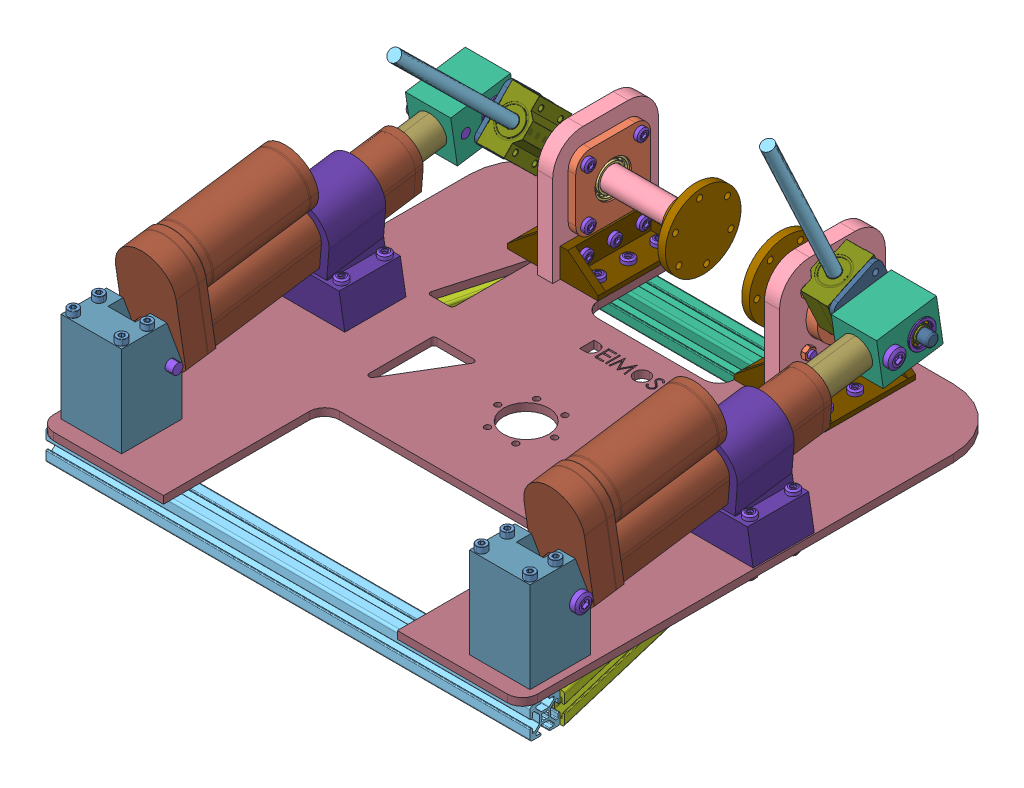
SolidWorks assembly Arm_base_2025_Final, configuration Default. Lengths in mm.
Overall size (325.65 204.06 325).
175 component instances, 27 part files, 250 mates.
Components (placement in the parent):
- linnear rod coupler-1: linnear rod coupler [Default] at (190.8714 137.6403 148.5796) x (0 0.712121 -0.702057) z (-1 0 0) size (18.5 18.5 20.01)
- base bearing assambly-1: base bearing assambly [Default] at (234.6957 114.573 126.7936) x (0 0 1) z (-1 0 0) size (49.5 49.5 22)
  - base shaft bearing housing-1: base shaft bearing housing [Default] at (21.786 23.0673 38.1242) size (49.5 49.5 22)
  - 61802  15x24x5mm-1: 61802  15x24x5mm [Default] at (21.786 23.0673 37.1242) x (0 0 -1) z (1 0 0) size (5 24 24)
  - 61802  15x24x5mm-2: 61802  15x24x5mm [Default] at (21.786 23.0673 22.1242) x (0 0 -1) z (1 0 0) size (5 24 24)
- V8_bearing holder holderURC 2024_V4-1: V8_bearing holder holderURC 2024_V4 [Default] at (213.5714 172.6403 113.5796) x (0 0 1) z (-1 0 0) size (70 80 10)
- linear guid rod-1: linear guid rod [Default] at (184.8714 141.8526 152.8523) x (0.966938 -0.1816 0.179034) z (-0.255013 -0.688576 0.678846) size (8 150 8)
- Connector to Linear bearing-1: Connector to Linear bearing [Default] at (123.1767 129.7873 154.7447) x (1 0 0) z (0 0.553629 0.832764) size (32.2 49.07 49.79)
  - V8_connectorURC 2024_V4-1: V8_connectorURC 2024_V4 [Default] at (40.3948 35.6094 31.6737) x (0 -0.66999 0.74237) z (-1 0 0) size (40 30 30)
  - V8_F688ZZ_assemblyURC 2024_V4-1: V8_F688ZZ_assemblyURC 2024_V4 [Default] at (41.4948 16.099 30.9035) x (0 1 0) z (0 0 1) size (20.89 5 20.89)
    - V8_F688ZZ_shaftURC 2024_V4-1: V8_F688ZZ_shaftURC 2024_V4 [Default] at origin size (10.7 5 10.7)
    - V8_F688ZZ_HousingURC 2024_V4-1: V8_F688ZZ_HousingURC 2024_V4 [Default] x (0.984312 0 0.176438) z (-0.176438 0 0.984312) size (18 5 18)
    - V8_F688ZZ_BallURC 2024_V4-1: V8_F688ZZ_BallURC 2024_V4 [Default] at (5.5752 2.5 -2.1489) x (0.959238 0.232099 0.161224) z (-0.142462 -0.095558 0.985177) size (2 2 2)
    - V8_F688ZZ_BallURC 2024_V4-20: V8_F688ZZ_BallURC 2024_V4 [Default] at (3.2474 2.5 -5.0155) x (0.870805 0.232099 -0.433393) z (0.463818 -0.095558 0.880762) size (2 2 2)
    - V8_F688ZZ_BallURC 2024_V4-21: V8_F688ZZ_BallURC 2024_V4 [Default] at (-0.3209 2.5 -5.9664) x (0.449753 0.232099 -0.862469) z (0.892936 -0.095558 0.439926) size (2 2 2)
    - V8_F688ZZ_BallURC 2024_V4-22: V8_F688ZZ_BallURC 2024_V4 [Default] at (-3.7665 2.5 -4.6383) x (-0.143088 0.232099 -0.96211) z (0.980982 -0.095558 -0.168947) size (2 2 2)
    - V8_F688ZZ_BallURC 2024_V4-23: V8_F688ZZ_BallURC 2024_V4 [Default] at (-5.7735 2.5 -1.5385) x (-0.681275 0.232099 -0.694258) z (0.694326 -0.095558 -0.713288) size (2 2 2)
    - V8_F688ZZ_BallURC 2024_V4-24: V8_F688ZZ_BallURC 2024_V4 [Default] at (-5.5752 2.5 2.1489) x (-0.959238 0.232099 -0.161224) z (0.142462 -0.095558 -0.985177) size (2 2 2)
    - V8_F688ZZ_BallURC 2024_V4-25: V8_F688ZZ_BallURC 2024_V4 [Default] at (-3.2474 2.5 5.0155) x (-0.870805 0.232099 0.433393) z (-0.463818 -0.095558 -0.880762) size (2 2 2)
    - V8_F688ZZ_BallURC 2024_V4-26: V8_F688ZZ_BallURC 2024_V4 [Default] at (0.3209 2.5 5.9664) x (-0.449753 0.232099 0.862469) z (-0.892936 -0.095558 -0.439926) size (2 2 2)
    - V8_F688ZZ_BallURC 2024_V4-27: V8_F688ZZ_BallURC 2024_V4 [Default] at (3.7665 2.5 4.6383) x (0.143088 0.232099 0.96211) z (-0.980982 -0.095558 0.168947) size (2 2 2)
    - V8_F688ZZ_BallURC 2024_V4-28: V8_F688ZZ_BallURC 2024_V4 [Default] at (5.7735 2.5 1.5385) x (0.681275 0.232099 0.694258) z (-0.694326 -0.095558 0.713288) size (2 2 2)
  - V8_F688ZZ_assemblyURC 2024_V4-2: V8_F688ZZ_assemblyURC 2024_V4 [Default] at (9.2948 16.099 30.9035) x (0 -0.381849 0.924225) z (0 0.924225 0.381849) size (20.89 5 20.89)
    - V8_F688ZZ_shaftURC 2024_V4-1: V8_F688ZZ_shaftURC 2024_V4 [Default] at origin size (10.7 5 10.7)
    - V8_F688ZZ_HousingURC 2024_V4-1: V8_F688ZZ_HousingURC 2024_V4 [Default] x (0.984312 0 0.176438) z (-0.176438 0 0.984312) size (18 5 18)
    - V8_F688ZZ_BallURC 2024_V4-1: V8_F688ZZ_BallURC 2024_V4 [Default] at (5.5752 2.5 -2.1489) x (0.959238 0.232099 0.161224) z (-0.142462 -0.095558 0.985177) size (2 2 2)
    - V8_F688ZZ_BallURC 2024_V4-20: V8_F688ZZ_BallURC 2024_V4 [Default] at (3.2474 2.5 -5.0155) x (0.870805 0.232099 -0.433393) z (0.463818 -0.095558 0.880762) size (2 2 2)
    - V8_F688ZZ_BallURC 2024_V4-21: V8_F688ZZ_BallURC 2024_V4 [Default] at (-0.3209 2.5 -5.9664) x (0.449753 0.232099 -0.862469) z (0.892936 -0.095558 0.439926) size (2 2 2)
    - V8_F688ZZ_BallURC 2024_V4-22: V8_F688ZZ_BallURC 2024_V4 [Default] at (-3.7665 2.5 -4.6383) x (-0.143088 0.232099 -0.96211) z (0.980982 -0.095558 -0.168947) size (2 2 2)
    - V8_F688ZZ_BallURC 2024_V4-23: V8_F688ZZ_BallURC 2024_V4 [Default] at (-5.7735 2.5 -1.5385) x (-0.681275 0.232099 -0.694258) z (0.694326 -0.095558 -0.713288) size (2 2 2)
    - V8_F688ZZ_BallURC 2024_V4-24: V8_F688ZZ_BallURC 2024_V4 [Default] at (-5.5752 2.5 2.1489) x (-0.959238 0.232099 -0.161224) z (0.142462 -0.095558 -0.985177) size (2 2 2)
    - V8_F688ZZ_BallURC 2024_V4-25: V8_F688ZZ_BallURC 2024_V4 [Default] at (-3.2474 2.5 5.0155) x (-0.870805 0.232099 0.433393) z (-0.463818 -0.095558 -0.880762) size (2 2 2)
    - V8_F688ZZ_BallURC 2024_V4-26: V8_F688ZZ_BallURC 2024_V4 [Default] at (0.3209 2.5 5.9664) x (-0.449753 0.232099 0.862469) z (-0.892936 -0.095558 -0.439926) size (2 2 2)
    - V8_F688ZZ_BallURC 2024_V4-27: V8_F688ZZ_BallURC 2024_V4 [Default] at (3.7665 2.5 4.6383) x (0.143088 0.232099 0.96211) z (-0.980982 -0.095558 0.168947) size (2 2 2)
    - V8_F688ZZ_BallURC 2024_V4-28: V8_F688ZZ_BallURC 2024_V4 [Default] at (5.7735 2.5 1.5385) x (0.681275 0.232099 0.694258) z (-0.694326 -0.095558 0.713288) size (2 2 2)
- V8_bearing and cam connection_for_v4URC 2024_V4 laser cut-1: V8_bearing and cam connection_for_v4URC 2024_V4 laser cut [Default] at (170.6714 137.31 173.1714) x (0 0.702057 0.712121) z (1 0 0) size (30 35 48)
- V8_LA_Body_V4-1: V8_LA_Body_V4 [Default] at (148.5714 135.8868 383.5572) x (0 -0.989144 -0.146946) z (-1 0 0) size (74 184 40)
- V8_LA_RodURC 2024_V4-1: V8_LA_RodURC 2024_V4 [Default] at (148.5714 158.4515 184.0304) x (1 0 0) z (0 -0.989144 -0.146946) size (20 121 20)
- V8_base plate for LAURC 2024_V4-1: V8_base plate for LAURC 2024_V4 [Default] at (283.5714 87.6403 412.2334) x (0 0 -1) z (0 1 0) size (325 320 5)
- LA_back holder-1: LA_back holder [Default] at (148.5714 152.6403 403.5796) x (-1 0 0) z (0 0 -1) size (40 60 40)
- Connector to Linear bearing-2: Connector to Linear bearing [Default] at (393.1767 131.5103 143.1465) x (1 0 0) z (0 0.553629 0.832764) size (32.2 49.07 49.79)
  - V8_connectorURC 2024_V4-1: V8_connectorURC 2024_V4 [Default] at (40.3948 35.6094 31.6737) x (0 -0.66999 0.74237) z (-1 0 0) size (40 30 30)
  - V8_F688ZZ_assemblyURC 2024_V4-1: V8_F688ZZ_assemblyURC 2024_V4 [Default] at (41.4948 16.099 30.9035) x (0 1 0) z (0 0 1) size (20.89 5 20.89)
    - V8_F688ZZ_shaftURC 2024_V4-1: V8_F688ZZ_shaftURC 2024_V4 [Default] at origin size (10.7 5 10.7)
    - V8_F688ZZ_HousingURC 2024_V4-1: V8_F688ZZ_HousingURC 2024_V4 [Default] x (0.984312 0 0.176438) z (-0.176438 0 0.984312) size (18 5 18)
    - V8_F688ZZ_BallURC 2024_V4-1: V8_F688ZZ_BallURC 2024_V4 [Default] at (5.5752 2.5 -2.1489) x (0.959238 0.232099 0.161224) z (-0.142462 -0.095558 0.985177) size (2 2 2)
    - V8_F688ZZ_BallURC 2024_V4-20: V8_F688ZZ_BallURC 2024_V4 [Default] at (3.2474 2.5 -5.0155) x (0.870805 0.232099 -0.433393) z (0.463818 -0.095558 0.880762) size (2 2 2)
    - V8_F688ZZ_BallURC 2024_V4-21: V8_F688ZZ_BallURC 2024_V4 [Default] at (-0.3209 2.5 -5.9664) x (0.449753 0.232099 -0.862469) z (0.892936 -0.095558 0.439926) size (2 2 2)
    - V8_F688ZZ_BallURC 2024_V4-22: V8_F688ZZ_BallURC 2024_V4 [Default] at (-3.7665 2.5 -4.6383) x (-0.143088 0.232099 -0.96211) z (0.980982 -0.095558 -0.168947) size (2 2 2)
    - V8_F688ZZ_BallURC 2024_V4-23: V8_F688ZZ_BallURC 2024_V4 [Default] at (-5.7735 2.5 -1.5385) x (-0.681275 0.232099 -0.694258) z (0.694326 -0.095558 -0.713288) size (2 2 2)
    - V8_F688ZZ_BallURC 2024_V4-24: V8_F688ZZ_BallURC 2024_V4 [Default] at (-5.5752 2.5 2.1489) x (-0.959238 0.232099 -0.161224) z (0.142462 -0.095558 -0.985177) size (2 2 2)
    - V8_F688ZZ_BallURC 2024_V4-25: V8_F688ZZ_BallURC 2024_V4 [Default] at (-3.2474 2.5 5.0155) x (-0.870805 0.232099 0.433393) z (-0.463818 -0.095558 -0.880762) size (2 2 2)
    - V8_F688ZZ_BallURC 2024_V4-26: V8_F688ZZ_BallURC 2024_V4 [Default] at (0.3209 2.5 5.9664) x (-0.449753 0.232099 0.862469) z (-0.892936 -0.095558 -0.439926) size (2 2 2)
    - V8_F688ZZ_BallURC 2024_V4-27: V8_F688ZZ_BallURC 2024_V4 [Default] at (3.7665 2.5 4.6383) x (0.143088 0.232099 0.96211) z (-0.980982 -0.095558 0.168947) size (2 2 2)
    - V8_F688ZZ_BallURC 2024_V4-28: V8_F688ZZ_BallURC 2024_V4 [Default] at (5.7735 2.5 1.5385) x (0.681275 0.232099 0.694258) z (-0.694326 -0.095558 0.713288) size (2 2 2)
  - V8_F688ZZ_assemblyURC 2024_V4-2: V8_F688ZZ_assemblyURC 2024_V4 [Default] at (9.2948 16.099 30.9035) x (0 -0.381849 0.924225) z (0 0.924225 0.381849) size (20.89 5 20.89)
    - V8_F688ZZ_shaftURC 2024_V4-1: V8_F688ZZ_shaftURC 2024_V4 [Default] at origin size (10.7 5 10.7)
    - V8_F688ZZ_HousingURC 2024_V4-1: V8_F688ZZ_HousingURC 2024_V4 [Default] x (0.984312 0 0.176438) z (-0.176438 0 0.984312) size (18 5 18)
    - V8_F688ZZ_BallURC 2024_V4-1: V8_F688ZZ_BallURC 2024_V4 [Default] at (5.5752 2.5 -2.1489) x (0.959238 0.232099 0.161224) z (-0.142462 -0.095558 0.985177) size (2 2 2)
    - V8_F688ZZ_BallURC 2024_V4-20: V8_F688ZZ_BallURC 2024_V4 [Default] at (3.2474 2.5 -5.0155) x (0.870805 0.232099 -0.433393) z (0.463818 -0.095558 0.880762) size (2 2 2)
    - V8_F688ZZ_BallURC 2024_V4-21: V8_F688ZZ_BallURC 2024_V4 [Default] at (-0.3209 2.5 -5.9664) x (0.449753 0.232099 -0.862469) z (0.892936 -0.095558 0.439926) size (2 2 2)
    - V8_F688ZZ_BallURC 2024_V4-22: V8_F688ZZ_BallURC 2024_V4 [Default] at (-3.7665 2.5 -4.6383) x (-0.143088 0.232099 -0.96211) z (0.980982 -0.095558 -0.168947) size (2 2 2)
    - V8_F688ZZ_BallURC 2024_V4-23: V8_F688ZZ_BallURC 2024_V4 [Default] at (-5.7735 2.5 -1.5385) x (-0.681275 0.232099 -0.694258) z (0.694326 -0.095558 -0.713288) size (2 2 2)
    - V8_F688ZZ_BallURC 2024_V4-24: V8_F688ZZ_BallURC 2024_V4 [Default] at (-5.5752 2.5 2.1489) x (-0.959238 0.232099 -0.161224) z (0.142462 -0.095558 -0.985177) size (2 2 2)
    - V8_F688ZZ_BallURC 2024_V4-25: V8_F688ZZ_BallURC 2024_V4 [Default] at (-3.2474 2.5 5.0155) x (-0.870805 0.232099 0.433393) z (-0.463818 -0.095558 -0.880762) size (2 2 2)
    - V8_F688ZZ_BallURC 2024_V4-26: V8_F688ZZ_BallURC 2024_V4 [Default] at (0.3209 2.5 5.9664) x (-0.449753 0.232099 0.862469) z (-0.892936 -0.095558 -0.439926) size (2 2 2)
    - V8_F688ZZ_BallURC 2024_V4-27: V8_F688ZZ_BallURC 2024_V4 [Default] at (3.7665 2.5 4.6383) x (0.143088 0.232099 0.96211) z (-0.980982 -0.095558 0.168947) size (2 2 2)
    - V8_F688ZZ_BallURC 2024_V4-28: V8_F688ZZ_BallURC 2024_V4 [Default] at (5.7735 2.5 1.5385) x (0.681275 0.232099 0.694258) z (-0.694326 -0.095558 0.713288) size (2 2 2)
- LA_back holder-2: LA_back holder [Default] at (418.5714 152.6403 403.5796) x (-1 0 0) z (0 0 -1) size (40 60 40)
- V8_bearing and cam connection_for_v4URC 2024_V4 laser cut-2: V8_bearing and cam connection_for_v4URC 2024_V4 laser cut [Default] at (396.4714 168.2112 182.1724) x (0 -0.906049 -0.423172) z (-1 0 0) size (30 35 48)
- V8_LA_RodURC 2024_V4-2: V8_LA_RodURC 2024_V4 [Default] at (418.5714 160.1745 172.4322) x (1 0 0) z (0 -0.989144 -0.146946) size (20 121 20)
- linnear rod coupler-2: linnear rod coupler [Default] at (376.2714 137.6403 148.5796) x (0 -0.423172 0.906049) z (1 0 0) size (18.5 18.5 20.01)
- lock_nut_for coupler-2: lock_nut_for coupler [Default] at (396.2714 137.6403 148.5796) x (0 -0.658716 -0.752392) z (1 0 0) size (18 18 13)
- linear guid rod-2: linear guid rod [Default] at (382.2714 133.5883 146.6871) x (0.37331 0.39258 -0.840548) z (0.927707 -0.157974 0.338237) size (8 150 8)
- base bearing assambly-2: base bearing assambly [Default] at (332.4472 114.573 170.3656) x (0 0 -1) z (1 0 0) size (49.5 49.5 22)
  - base shaft bearing housing-1: base shaft bearing housing [Default] at (21.786 23.0673 38.1242) size (49.5 49.5 22)
  - 61802  15x24x5mm-1: 61802  15x24x5mm [Default] at (21.786 23.0673 37.1242) x (0 0 -1) z (1 0 0) size (5 24 24)
  - 61802  15x24x5mm-2: 61802  15x24x5mm [Default] at (21.786 23.0673 22.1242) x (0 0 -1) z (1 0 0) size (5 24 24)
- V8_bearing holder holderURC 2024_V4-2: V8_bearing holder holderURC 2024_V4 [Default] at (353.5714 172.6403 183.5796) x (0 0 -1) z (1 0 0) size (70 80 10)
- V8_LA_Body_V4-2: V8_LA_Body_V4 [Default] at (418.5714 135.8868 383.5572) x (0 -0.989144 -0.146946) z (-1 0 0) size (74 184 40)
- linear bearing robotic arm-1: linear bearing robotic arm [Default] at (182.4393 149.7722 160.8854) x (0 0.712121 -0.702057) z (1 0 0) size (34 30.1 22.2)
- linear bearing robotic arm-2: linear bearing robotic arm [Default] at (384.7035 175.6167 166.3166) x (0 0.423172 -0.906049) z (-1 0 0) size (34 30.1 22.2)
- linear_acutator_holder-1: linear_acutator_holder [Default] at (418.6971 146.656 247.7322) x (0 -0.989144 -0.146946) z (0 -0.146946 0.989144) size (75.87 48 40)
- linear_acutator_holder-2: linear_acutator_holder [Default] at (148.6971 146.656 247.7322) x (0 -0.989144 -0.146946) z (0 -0.146946 0.989144) size (75.87 48 40)
- l bracket_arm base flang-1: l bracket_arm base flang [Default] at (363.5714 111.6403 178.5796) x (0 0 -1) z (1 0 0) size (60 19 25)
- l bracket_arm base flang-2: l bracket_arm base flang [Default] at (353.5714 111.6403 118.5796) x (0 0 1) z (-1 0 0) size (60 19 25)
- l bracket_arm base flang-3: l bracket_arm base flang [Default] at (203.5714 111.6403 118.5796) x (0 0 1) z (-1 0 0) size (60 19 25)
- l bracket_arm base flang-4: l bracket_arm base flang [Default] at (213.5714 111.6403 178.5796) x (0 0 -1) z (1 0 0) size (60 19 25)
- Screw_DIN_912_M4x70_A2.step-1: Screw_DIN_912_M4x70_A2.step [Default] at (402.5714 82.6403 419.5796) size (7 74 7)
- Screw_DIN_912_M4x70_A2.step-2: Screw_DIN_912_M4x70_A2.step [Default] at (434.5714 82.6403 419.5796) x (0.982082 0 -0.188455) z (0.188455 0 0.982082) size (7 74 7)
- Screw_DIN_912_M4x70_A2.step-4: Screw_DIN_912_M4x70_A2.step [Default] at (434.5714 82.6403 402.6026) x (0.918365 0 -0.395734) z (0.395734 0 0.918365) size (7 74 7)
- Screw_DIN_912_M4x70_A2.step-6: Screw_DIN_912_M4x70_A2.step [Default] at (402.5714 82.6403 402.6026) x (0.8 0 -0.6) z (0.6 0 0.8) size (7 74 7)
- Screw_DIN_912_M4x70_A2.step-8: Screw_DIN_912_M4x70_A2.step [Default] at (164.5714 82.6403 419.5796) x (0.63358 0 -0.773678) z (0.773678 0 0.63358) size (7 74 7)
- Screw_DIN_912_M4x70_A2.step-10: Screw_DIN_912_M4x70_A2.step [Default] at (164.5714 82.6403 402.6026) x (0.443629 0 -0.896211) z (0.896211 0 0.443629) size (7 74 7)
- Screw_DIN_912_M4x70_A2.step-12: Screw_DIN_912_M4x70_A2.step [Default] at (132.5714 82.6403 419.5796) x (0.263225 0 -0.964735) z (0.964735 0 0.263225) size (7 74 7)
- Screw_DIN_912_M4x70_A2.step-14: Screw_DIN_912_M4x70_A2.step [Default] at (132.5714 82.6403 402.6026) x (0.120178 0 -0.992752) z (0.992752 0 0.120178) size (7 74 7)
- hex nut style 1 gradeab_iso-8: hex nut style 1 gradeab_iso [ISO - 4032 - M4 - W - N] at (402.5714 84.4403 419.5796) x (0.999814 0 0.019309) z (0 -1 0) size (7 8.08 3.2)
- hex nut style 1 gradeab_iso-9: hex nut style 1 gradeab_iso [ISO - 4032 - M4 - W - N] at (434.5714 84.4403 419.5796) x (0.985538 0 -0.169457) z (0 -1 0) size (7 8.08 3.2)
- hex nut style 1 gradeab_iso-11: hex nut style 1 gradeab_iso [ISO - 4032 - M4 - W - N] at (434.5714 84.4403 402.6026) x (0.563007 0 -0.826452) z (0 -1 0) size (7 8.08 3.2)
- hex nut style 1 gradeab_iso-14: hex nut style 1 gradeab_iso [ISO - 4032 - M4 - W - N] at (402.5714 84.4403 402.6026) x (0.563007 0 -0.826452) z (0 -1 0) size (7 8.08 3.2)
- hex nut style 1 gradeab_iso-16: hex nut style 1 gradeab_iso [ISO - 4032 - M4 - W - N] at (164.5714 84.4403 419.5796) x (0.648401 0 -0.761299) z (0 -1 0) size (7 8.08 3.2)
- hex nut style 1 gradeab_iso-18: hex nut style 1 gradeab_iso [ISO - 4032 - M4 - W - N] at (164.5714 84.4403 402.6026) x (0.563007 0 -0.826452) z (0 -1 0) size (7 8.08 3.2)
- hex nut style 1 gradeab_iso-20: hex nut style 1 gradeab_iso [ISO - 4032 - M4 - W - N] at (132.5714 84.4403 419.5796) x (0.563007 0 -0.826452) z (0 -1 0) size (7 8.08 3.2)
- hex nut style 1 gradeab_iso-22: hex nut style 1 gradeab_iso [ISO - 4032 - M4 - W - N] at (132.5714 84.4403 402.6026) x (0.563007 0 -0.826452) z (0 -1 0) size (7 8.08 3.2)
- V8_shaftURC 2024_V4 real part-1: V8_shaftURC 2024_V4 real part [Default] at (378.5714 128.7575 141.4959) x (-1 0 0) z (0 0.623486 -0.781835) size (75.7 15 15)
- V8_shaftURC 2024_V4-1: V8_shaftURC 2024_V4 [Default] at (223.809 124.5508 145.7858) x (1 0 0) z (0 -0.208738 0.977971) size (115.2 15 15)
- 20 20 aluminium extrusion T slot-1: 20 20 aluminium extrusion T slot [Default] at (4123.5714 77.6403 418.5796) x (0 0 -1) z (-1 0 0) size (20 20 320)
- 20 20 aluminium extrusion T slot 200 mm-1: 20 20 aluminium extrusion T slot 200 mm [Default] at (4183.5714 77.6403 148.5796) x (0 0 -1) z (-1 0 0) size (20 20 200)
- 20 20 aluminium extrusion T slot at angle-1: 20 20 aluminium extrusion T slot at angle [Default] at (-494.3957 77.6403 -3479.2697) x (0.972533 0 -0.232766) z (0.232766 0 0.972533) size (20 20 261.8)
- 20 20 aluminium extrusion T slot at angle-2: 20 20 aluminium extrusion T slot at angle [Default] at (-739.6549 77.6403 4046.3826) x (0.972533 0 0.232766) z (0.232766 0 -0.972533) size (20 20 261.8)
- hexalobular socket pan head_iso-2: hexalobular socket pan head_iso [ISO 14583 - M4 x 12 x 10.6 - 4.8-N] at (378.5714 83.6403 168.5796) size (8 15.1 8)
- hexalobular socket pan head_iso-3: hexalobular socket pan head_iso [ISO 14583 - M4 x 12 x 10.6 - 4.8-N] at (378.5714 83.6403 148.5796) size (8 15.1 8)
- hexalobular socket pan head_iso-4: hexalobular socket pan head_iso [ISO 14583 - M4 x 12 x 10.6 - 4.8-N] at (378.5714 83.6403 128.5796) size (8 15.1 8)
- hexalobular socket pan head_iso-5: hexalobular socket pan head_iso [ISO 14583 - M4 x 12 x 10.6 - 4.8-N] at (338.5714 83.6403 168.5796) size (8 15.1 8)
- hexalobular socket pan head_iso-6: hexalobular socket pan head_iso [ISO 14583 - M4 x 12 x 10.6 - 4.8-N] at (338.5714 83.6403 148.5796) size (8 15.1 8)
- hexalobular socket pan head_iso-7: hexalobular socket pan head_iso [ISO 14583 - M4 x 12 x 10.6 - 4.8-N] at (338.5714 83.6403 128.5796) size (8 15.1 8)
- hexalobular socket pan head_iso-8: hexalobular socket pan head_iso [ISO 14583 - M4 x 12 x 10.6 - 4.8-N] at (228.5714 83.6403 128.5796) size (8 15.1 8)
- hexalobular socket pan head_iso-9: hexalobular socket pan head_iso [ISO 14583 - M4 x 12 x 10.6 - 4.8-N] at (228.5714 83.6403 148.5796) size (8 15.1 8)
- hexalobular socket pan head_iso-10: hexalobular socket pan head_iso [ISO 14583 - M4 x 12 x 10.6 - 4.8-N] at (228.5714 83.6403 168.5796) size (8 15.1 8)
- hexalobular socket pan head_iso-11: hexalobular socket pan head_iso [ISO 14583 - M4 x 12 x 10.6 - 4.8-N] at (188.5714 83.6403 128.5796) size (8 15.1 8)
- hexalobular socket pan head_iso-12: hexalobular socket pan head_iso [ISO 14583 - M4 x 12 x 10.6 - 4.8-N] at (188.5714 83.6403 148.5796) size (8 15.1 8)
- hexalobular socket pan head_iso-13: hexalobular socket pan head_iso [ISO 14583 - M4 x 12 x 10.6 - 4.8-N] at (188.5714 83.6403 168.5796) size (8 15.1 8)
- hexalobular socket pan head_iso-16: hexalobular socket pan head_iso [ISO 14583 - M4 x 25 x 23.6 - 4.8-N] at (373.5714 103.6403 129.5796) x (0 1 0) z (0 0 1) size (8 28.1 8)
- hexalobular socket pan head_iso-17: hexalobular socket pan head_iso [ISO 14583 - M4 x 25 x 23.6 - 4.8-N] at (373.5714 103.6403 148.5796) x (0 1 0) z (0 0 1) size (8 28.1 8)
- hexalobular socket pan head_iso-18: hexalobular socket pan head_iso [ISO 14583 - M4 x 25 x 23.6 - 4.8-N] at (373.5714 103.6403 167.5796) x (0 1 0) z (0 0 1) size (8 28.1 8)
- hexalobular socket pan head_iso-19: hexalobular socket pan head_iso [ISO 14583 - M4 x 25 x 23.6 - 4.8-N] at (193.5714 103.6403 167.5796) x (0 -1 0) z (0 0 1) size (8 28.1 8)
- hexalobular socket pan head_iso-20: hexalobular socket pan head_iso [ISO 14583 - M4 x 25 x 23.6 - 4.8-N] at (193.5714 103.6403 148.5796) x (0 -1 0) z (0 0 1) size (8 28.1 8)
- hexalobular socket pan head_iso-21: hexalobular socket pan head_iso [ISO 14583 - M4 x 25 x 23.6 - 4.8-N] at (193.5714 103.6403 129.5796) x (0 -1 0) z (0 0 1) size (8 28.1 8)
- hexalobular socket pan head_iso-23: hexalobular socket pan head_iso [ISO 14583 - M4 x 20 x 18.6 - 4.8-N] at (368.5714 155.1403 131.0796) x (0 1 0) z (0 0 1) size (8 23.1 8)
- hexalobular socket pan head_iso-24: hexalobular socket pan head_iso [ISO 14583 - M4 x 20 x 18.6 - 4.8-N] at (368.5714 155.1403 166.0796) x (0 1 0) z (0 0 1) size (8 23.1 8)
- hexalobular socket pan head_iso-25: hexalobular socket pan head_iso [ISO 14583 - M4 x 20 x 18.6 - 4.8-N] at (368.5714 120.1403 131.0796) x (0 1 0) z (0 0 1) size (8 23.1 8)
- hexalobular socket pan head_iso-26: hexalobular socket pan head_iso [ISO 14583 - M4 x 20 x 18.6 - 4.8-N] at (368.5714 120.1403 166.0796) x (0 1 0) z (0 0 1) size (8 23.1 8)
- hexalobular socket pan head_iso-27: hexalobular socket pan head_iso [ISO 14583 - M4 x 20 x 18.6 - 4.8-N] at (198.5714 120.1403 131.0796) x (0 -1 0) z (0 0 1) size (8 23.1 8)
- hexalobular socket pan head_iso-28: hexalobular socket pan head_iso [ISO 14583 - M4 x 20 x 18.6 - 4.8-N] at (198.5714 155.1403 131.0796) x (0 -1 0) z (0 0 1) size (8 23.1 8)
- hexalobular socket pan head_iso-29: hexalobular socket pan head_iso [ISO 14583 - M4 x 20 x 18.6 - 4.8-N] at (198.5714 155.1403 166.0796) x (0 -1 0) z (0 0 1) size (8 23.1 8)
- hexalobular socket pan head_iso-30: hexalobular socket pan head_iso [ISO 14583 - M4 x 20 x 18.6 - 4.8-N] at (198.5714 120.1403 166.0796) x (0 -1 0) z (0 0 1) size (8 23.1 8)
- hexalobular socket pan head_iso-32: hexalobular socket pan head_iso [ISO 14583 - M4 x 35 x 33.6 - 4.8-N] at (437.6971 83.0703 277.3153) size (8 38.1 8)
- hexalobular socket pan head_iso-33: hexalobular socket pan head_iso [ISO 14583 - M4 x 35 x 33.6 - 4.8-N] at (437.6971 83.0703 248.7068) size (8 38.1 8)
- hexalobular socket pan head_iso-34: hexalobular socket pan head_iso [ISO 14583 - M4 x 35 x 33.6 - 4.8-N] at (399.6971 83.0703 277.3153) size (8 38.1 8)
- hexalobular socket pan head_iso-35: hexalobular socket pan head_iso [ISO 14583 - M4 x 35 x 33.6 - 4.8-N] at (399.6971 83.0703 248.7068) size (8 38.1 8)
- hexalobular socket pan head_iso-36: hexalobular socket pan head_iso [ISO 14583 - M4 x 35 x 33.6 - 4.8-N] at (129.6971 83.0703 248.7068) size (8 38.1 8)
- hexalobular socket pan head_iso-37: hexalobular socket pan head_iso [ISO 14583 - M4 x 35 x 33.6 - 4.8-N] at (129.6971 83.0703 277.3153) size (8 38.1 8)
- hexalobular socket pan head_iso-38: hexalobular socket pan head_iso [ISO 14583 - M4 x 35 x 33.6 - 4.8-N] at (167.6971 83.0703 248.7068) size (8 38.1 8)
- hexalobular socket pan head_iso-39: hexalobular socket pan head_iso [ISO 14583 - M4 x 35 x 33.6 - 4.8-N] at (167.6971 83.0703 277.3153) size (8 38.1 8)
- hexalobular socket pan head_iso-41: hexalobular socket pan head_iso [ISO 14583 - M6 x 30 x 28 - 4.8-N] at (163.5714 157.4228 190.9544) x (0 1 0) z (0 0 1) size (12 34.6 12)
- hexalobular socket pan head_iso-42: hexalobular socket pan head_iso [ISO 14583 - M6 x 30 x 28 - 4.8-N] at (403.5714 159.1459 179.3562) x (0 -1 0) z (0 0 1) size (12 34.6 12)
- hex nut style 1 gradeab_iso-24: hex nut style 1 gradeab_iso [ISO - 4032 - M4 - W - N] at (371.7714 103.6403 148.5796) x (0 0.916221 0.400674) z (1 0 0) size (7 8.08 3.2)
- hex nut style 1 gradeab_iso-25: hex nut style 1 gradeab_iso [ISO - 4032 - M4 - W - N] at (371.7714 103.6403 167.5796) x (0 0 -1) z (1 0 0) size (7 8.08 3.2)
- hex nut style 1 gradeab_iso-26: hex nut style 1 gradeab_iso [ISO - 4032 - M4 - W - N] at (371.7714 103.6403 129.5796) x (0 0 -1) z (1 0 0) size (7 8.08 3.2)
- hex nut style 1 gradeab_iso-27: hex nut style 1 gradeab_iso [ISO - 4032 - M4 - W - N] at (366.7714 120.1403 131.0796) x (0 0 -1) z (1 0 0) size (7 8.08 3.2)
- hex nut style 1 gradeab_iso-28: hex nut style 1 gradeab_iso [ISO - 4032 - M4 - W - N] at (366.7714 155.1403 131.0796) x (0 0.719892 -0.694086) z (1 0 0) size (7 8.08 3.2)
- hex nut style 1 gradeab_iso-29: hex nut style 1 gradeab_iso [ISO - 4032 - M4 - W - N] at (366.7714 155.1403 166.0796) x (0 0 -1) z (1 0 0) size (7 8.08 3.2)
- hex nut style 1 gradeab_iso-30: hex nut style 1 gradeab_iso [ISO - 4032 - M4 - W - N] at (378.5714 84.4403 128.5796) x (1 0 0) z (0 -1 0) size (7 8.08 3.2)
- hex nut style 1 gradeab_iso-31: hex nut style 1 gradeab_iso [ISO - 4032 - M4 - W - N] at (338.5714 84.4403 128.5796) x (1 0 0) z (0 -1 0) size (7 8.08 3.2)
- hex nut style 1 gradeab_iso-32: hex nut style 1 gradeab_iso [ISO - 4032 - M4 - W - N] at (338.5714 84.4403 168.5796) x (1 0 0) z (0 -1 0) size (7 8.08 3.2)
- hex nut style 1 gradeab_iso-34: hex nut style 1 gradeab_iso [ISO - 4032 - M4 - W - N] at (366.7714 120.1403 166.0796) x (0 0 -1) z (1 0 0) size (7 8.08 3.2)
- hex nut style 1 gradeab_iso-35: hex nut style 1 gradeab_iso [ISO - 4032 - M4 - W - N] at (200.3714 155.1403 131.0796) x (0 0 1) z (-1 0 0) size (7 8.08 3.2)
- hex nut style 1 gradeab_iso-36: hex nut style 1 gradeab_iso [ISO - 4032 - M4 - W - N] at (200.3714 120.1403 131.0796) x (0 0 1) z (-1 0 0) size (7 8.08 3.2)
- hex nut style 1 gradeab_iso-37: hex nut style 1 gradeab_iso [ISO - 4032 - M4 - W - N] at (200.3714 155.1403 166.0796) x (0 0 1) z (-1 0 0) size (7 8.08 3.2)
- hex nut style 1 gradeab_iso-38: hex nut style 1 gradeab_iso [ISO - 4032 - M4 - W - N] at (200.3714 120.1403 166.0796) x (0 0 1) z (-1 0 0) size (7 8.08 3.2)
- hex nut style 1 gradeab_iso-39: hex nut style 1 gradeab_iso [ISO - 4032 - M4 - W - N] at (195.3714 103.6403 148.5796) x (0 0 1) z (-1 0 0) size (7 8.08 3.2)
- hex nut style 1 gradeab_iso-40: hex nut style 1 gradeab_iso [ISO - 4032 - M4 - W - N] at (195.3714 103.6403 167.5796) x (0 0 1) z (-1 0 0) size (7 8.08 3.2)
- hex nut style 1 gradeab_iso-41: hex nut style 1 gradeab_iso [ISO - 4032 - M4 - W - N] at (195.3714 103.6403 129.5796) x (0 0 1) z (-1 0 0) size (7 8.08 3.2)
- hex nut style 1 gradeab_iso-42: hex nut style 1 gradeab_iso [ISO - 4032 - M4 - W - N] at (228.5714 84.4403 128.5796) x (1 0 0) z (0 -1 0) size (7 8.08 3.2)
- hex nut style 1 gradeab_iso-43: hex nut style 1 gradeab_iso [ISO - 4032 - M4 - W - N] at (188.5714 84.4403 128.5796) x (1 0 0) z (0 -1 0) size (7 8.08 3.2)
- hex nut style 1 gradeab_iso-44: hex nut style 1 gradeab_iso [ISO - 4032 - M4 - W - N] at (228.5714 84.4403 168.5796) x (1 0 0) z (0 -1 0) size (7 8.08 3.2)
- hex nut style 1 gradeab_iso-45: hex nut style 1 gradeab_iso [ISO - 4032 - M4 - W - N] at (129.6971 84.4403 277.3153) x (1 0 0) z (0 -1 0) size (7 8.08 3.2)
- hex nut style 1 gradeab_iso-46: hex nut style 1 gradeab_iso [ISO - 4032 - M4 - W - N] at (129.6971 84.4403 248.7068) x (1 0 0) z (0 -1 0) size (7 8.08 3.2)
- hex nut style 1 gradeab_iso-47: hex nut style 1 gradeab_iso [ISO - 4032 - M4 - W - N] at (437.6971 84.4403 277.3153) x (-0.32211 0 -0.946702) z (0 -1 0) size (7 8.08 3.2)
- hex nut style 1 gradeab_iso-48: hex nut style 1 gradeab_iso [ISO - 4032 - M4 - W - N] at (437.4458 84.4403 248.7068) x (0.082905 0 -0.996557) z (0 -1 0) size (7 8.08 3.2)
- hexalobular socket pan head_iso-44: hexalobular socket pan head_iso [ISO 14583 - M6 x 45 x 38 - 4.8-N] at (173.5714 127.6403 391.4309) x (0 1 0) z (0 0 1) size (12 49.6 12)
- hexalobular socket pan head_iso-45: hexalobular socket pan head_iso [ISO 14583 - M6 x 45 x 43 - 4.8-N] at (393.5714 127.6403 391.4309) x (0 -1 0) z (0 0 1) size (12 49.6 12)
- Base Shaft connector to link 1-1: Base Shaft connector to link 1 [Default] at (328.5714 137.6403 148.5796) x (0 -0.997764 -0.066837) z (1 0 0) size (50 50 15)
- lock_nut_for coupler-3: lock_nut_for coupler [Default] at (170.8714 137.6403 148.5796) x (0 0.443849 0.896102) z (-1 0 0) size (18 18 13)
- Base Shaft connector to link 1-2: Base Shaft connector to link 1 [Default] at (278.0714 137.6403 148.5796) x (0 -0.114715 0.993398) z (-1 0 0) size (50 50 15)
Mates (geometry in assembly coordinates):
- Coincident12: coincident anti-aligned: plane of V8_base plate for LAURC 2024_V4-1 through (283.5714 92.6403 412.2334) normal (0 1 0); plane of LA_back holder-1 through (148.5714 92.6403 403.5796) normal (0 -1 0)
- Concentric4: concentric anti-aligned: cylinder of Connector to Linear bearing-1/V8_F688ZZ_assemblyURC 2024_V4-2/V8_F688ZZ_shaftURC 2024_V4-1 through (137.4714 160.303 171.5672) axis (-1 0 0) radius 4; cylinder of V8_bearing and cam connection_for_v4URC 2024_V4 laser cut-1 through (125.6714 160.303 171.5672) axis (1 0 0) radius 4
- Distance6: distance = 20 mm: cylinder of Connector to Linear bearing-1/V8_connectorURC 2024_V4-1 through (168.5714 167.5156 156.635) axis (0 -0.146923 0.989148) radius 13; plane of V8_bearing and cam connection_for_v4URC 2024_V4-1 through (188.5714 161.6723 163.3962) normal (-1 0 0)
- Concentric7: concentric aligned: cylinder of V8_LA_Body_V4-1 through (148.5714 127.7454 390.7229) axis (0 0.146946 -0.989144) radius 10; cylinder of V8_LA_RodURC 2024_V4-1 through (148.5714 140.671 303.7169) axis (0 0.146946 -0.989144) radius 10
- Parallel7: parallel aligned: plane of V8_bearing and cam connection_for_v4URC 2024_V4 laser cut-1 through (170.6714 137.31 173.1714) normal (-1 0 0); plane of V8_base plate for LAURC 2024_V4-1 through (123.5714 92.6403 412.2334) normal (-1 0 0)
- Coincident16: coincident anti-aligned: plane of V8_LA_Body_V4-1 through (139.5714 133.2418 401.3618) normal (-1 0 0); plane of LA_back holder-1 through (139.5714 102.6403 403.5796) normal (1 0 0)
- Concentric13: concentric aligned: cylinder of V8_LA_Body_V4-1 through (166.0567 127.6403 391.4309) axis (-1 0 0) radius 3; cylinder of LA_back holder-1 through (196.5714 127.6403 391.4309) axis (-1 0 0) radius 3
- Concentric14: concentric aligned: cylinder of linnear rod coupler-1 through (184.8714 146.065 157.125) axis (0 -0.702057 -0.712121) radius 4; cylinder of linear guid rod-1 through (184.8714 247.1612 259.6704) axis (0 -0.702057 -0.712121) radius 4
- Concentric15: concentric: cylinder of base bearing assambly-1/base shaft bearing housing-1 through (214.5714 142.6403 150.9703) axis (-1 0 0) radius 17; cylinder of V8_bearing holder holderURC 2024_V4-1 through (223.5714 142.6403 150.9703) axis (1 0 0) radius 17.5
- Coincident19: coincident anti-aligned: plane of V8_bearing holder holderURC 2024_V4-1 through (203.5714 92.6403 113.5796) normal (0 -1 0); plane of V8_base plate for LAURC 2024_V4-1 through (283.5714 92.6403 412.2334) normal (0 1 0)
- Concentric21: concentric aligned: cylinder of V8_LA_Body_V4-1 through (166.0567 127.6403 391.4309) axis (-1 0 0) radius 3; cylinder of LA_back holder-1 through (196.5714 127.6403 391.4309) axis (-1 0 0) radius 3
- Concentric24: concentric anti-aligned: cylinder of V8_base plate for LAURC 2024_V4-1 through (132.5714 82.6403 419.5796) axis (0 1 0) radius 2; cylinder of LA_back holder-1 through (132.5714 180.6403 419.5796) axis (0 -1 0) radius 2
- Concentric25: concentric anti-aligned: cylinder of V8_base plate for LAURC 2024_V4-1 through (164.5714 82.6403 419.5796) axis (0 1 0) radius 2; cylinder of LA_back holder-1 through (164.5714 180.6403 419.5796) axis (0 -1 0) radius 2
- Concentric26: concentric aligned: cylinder of Connector to Linear bearing-2/V8_F688ZZ_assemblyURC 2024_V4-2/V8_F688ZZ_shaftURC 2024_V4-1 through (407.4714 162.026 159.969) axis (-1 0 0) radius 4; cylinder of V8_bearing and cam connection_for_v4URC 2024_V4 laser cut-2 through (441.4714 162.026 159.969) axis (-1 0 0) radius 4
- Concentric31: concentric aligned: cylinder of V8_LA_RodURC 2024_V4-2 through (418.5714 142.394 292.1187) axis (0 0.146946 -0.989144) radius 10; cylinder of V8_LA_Body_V4-2 through (418.5714 127.7454 390.7229) axis (0 0.146946 -0.989144) radius 10
- Concentric36: concentric aligned: cylinder of linnear rod coupler-2 through (382.2714 148.5129 153.6577) axis (0 -0.906049 -0.423172) radius 4; cylinder of linear guid rod-2 through (382.2714 269.4957 210.1629) axis (0 -0.906049 -0.423172) radius 4
- Concentric37: concentric anti-aligned: cylinder of base bearing assambly-2/base shaft bearing housing-1 through (370.5714 137.6403 148.5796) axis (1 0 0) radius 17; cylinder of V8_bearing holder holderURC 2024_V4-2 through (363.5714 137.6403 148.5796) axis (-1 0 0) radius 17.5
- Coincident30: coincident anti-aligned: plane of linnear rod coupler-2 through (396.2714 137.6403 148.5796) normal (1 0 0); plane of lock_nut_for coupler-2 through (396.2714 137.6403 148.5796) normal (-1 0 0)
- Coincident31: coincident anti-aligned: plane of V8_base plate for LAURC 2024_V4-1 through (283.5714 92.6403 412.2334) normal (0 1 0); plane of LA_back holder-2 through (418.5714 92.6403 403.5796) normal (0 -1 0)
- Parallel13: parallel aligned: plane of V8_base plate for LAURC 2024_V4-1 through (443.5714 92.6403 412.2334) normal (1 0 0); plane of V8_bearing and cam connection_for_v4URC 2024_V4 laser cut-2 through (396.4714 168.2112 182.1724) normal (1 0 0)
- Coincident32: coincident anti-aligned: plane of V8_base plate for LAURC 2024_V4-1 through (283.5714 92.6403 412.2334) normal (0 1 0); plane of V8_bearing holder holderURC 2024_V4-2 through (363.5714 92.6403 183.5796) normal (0 -1 0)
- Concentric42: concentric anti-aligned: cylinder of V8_base plate for LAURC 2024_V4-1 through (402.5714 82.6403 419.5796) axis (0 1 0) radius 2; cylinder of LA_back holder-2 through (402.5714 180.6403 419.5796) axis (0 -1 0) radius 2
- Concentric43: concentric anti-aligned: cylinder of V8_base plate for LAURC 2024_V4-1 through (434.5714 82.6403 419.5796) axis (0 1 0) radius 2; cylinder of LA_back holder-2 through (434.5714 180.6403 419.5796) axis (0 -1 0) radius 2
- Coincident41: coincident anti-aligned: plane of LA_back holder-2 through (427.5714 102.6403 403.5796) normal (-1 0 0); plane of V8_LA_Body_V4-2 through (427.5714 133.2418 401.3618) normal (1 0 0)
- Concentric60: concentric aligned: cylinder of LA_back holder-2 through (466.5714 127.6403 391.4309) axis (-1 0 0) radius 3; cylinder of V8_LA_Body_V4-2 through (436.0567 127.6403 391.4309) axis (-1 0 0) radius 3
- Coincident46: coincident anti-aligned: plane of V8_bearing and cam connection_for_v4URC 2024_V4 laser cut-2 through (393.4714 168.2112 182.1724) normal (-1 0 0); plane of linear bearing robotic arm-2 through (393.4714 185.0413 170.7184) normal (1 0 0)
- Concentric65: concentric anti-aligned: cylinder of V8_bearing and cam connection_for_v4URC 2024_V4 laser cut-2 through (403.4714 148.7935 167.033) axis (-1 0 0) radius 2; cylinder of linear bearing robotic arm-2 through (385.4714 148.7935 167.033) axis (1 0 0) radius 1.7
- Concentric66: concentric anti-aligned: cylinder of V8_bearing and cam connection_for_v4URC 2024_V4 laser cut-2 through (403.4714 165.1024 174.6501) axis (-1 0 0) radius 2; cylinder of linear bearing robotic arm-2 through (385.4714 165.1024 174.6501) axis (1 0 0) radius 1.7
- Coincident47: coincident anti-aligned: plane of V8_bearing and cam connection_for_v4URC 2024_V4 laser cut-1 through (173.6714 137.31 173.1714) normal (1 0 0); plane of linear bearing robotic arm-1 through (173.6714 142.4694 153.478) normal (-1 0 0)
- Concentric67: concentric aligned: cone of V8_bearing and cam connection_for_v4URC 2024_V4 laser cut-1 through (163.6714 175.167 169.5516) axis (1 0 0); cylinder of linear bearing robotic arm-1 through (173.7714 175.167 169.5516) axis (1 0 0) radius 785.3982
- Concentric68: concentric aligned: cylinder of V8_bearing and cam connection_for_v4URC 2024_V4 laser cut-1 through (163.6714 162.5299 156.7334) axis (1 0 0) radius 2; cylinder of linear bearing robotic arm-1 through (173.7714 162.5299 156.7334) axis (1 0 0) radius 785.3982
- Concentric69: concentric anti-aligned: cylinder of linear guid rod-2 through (382.2714 269.4957 210.1629) axis (0 -0.906049 -0.423172) radius 4; cylinder of linear bearing robotic arm-2 through (382.2714 148.4352 153.6214) axis (0 0.906049 0.423172) radius 4
- Concentric70: concentric aligned: cylinder of linear guid rod-1 through (184.8714 247.1612 259.6704) axis (0 -0.702057 -0.712121) radius 4; cylinder of linear bearing robotic arm-1 through (184.8714 170.8339 182.249) axis (0 -0.702057 -0.712121) radius 4
- Concentric73: concentric anti-aligned: cylinder of V8_LA_Body_V4-2 through (418.5714 153.3559 218.3306) axis (0 -0.146946 0.989144) radius 14.0003; cylinder of linear_acutator_holder-1 through (418.5714 143.3537 285.6586) axis (0 0.146946 -0.989144) radius 13.9658
- Concentric74: concentric anti-aligned: cylinder of Connector to Linear bearing-2/V8_connectorURC 2024_V4-1 through (418.5714 160.1892 172.3333) axis (0 -0.146946 0.989144) radius 10; cylinder of V8_LA_RodURC 2024_V4-2 through (418.5714 142.394 292.1187) axis (0 0.146946 -0.989144) radius 10
- Concentric76: concentric anti-aligned: cylinder of Connector to Linear bearing-2/V8_connectorURC 2024_V4-1 through (504.5714 159.1459 179.3562) axis (-1 0 0) radius 3; cylinder of V8_LA_RodURC 2024_V4-2 through (408.5704 159.1459 179.3562) axis (1 0 0) radius 3
- Concentric77: concentric anti-aligned: cylinder of Connector to Linear bearing-1/V8_connectorURC 2024_V4-1 through (148.5714 158.4662 183.9315) axis (0 -0.146946 0.989144) radius 10; cylinder of V8_LA_RodURC 2024_V4-1 through (148.5714 140.671 303.7169) axis (0 0.146946 -0.989144) radius 10
- Concentric78: concentric anti-aligned: cylinder of Connector to Linear bearing-1/V8_connectorURC 2024_V4-1 through (234.5714 157.4228 190.9544) axis (-1 0 0) radius 3; cylinder of V8_LA_RodURC 2024_V4-1 through (138.5704 157.4228 190.9544) axis (1 0 0) radius 3
- Coincident51: coincident anti-aligned: plane of V8_base plate for LAURC 2024_V4-1 through (283.5714 92.6403 412.2334) normal (0 1 0); plane of linear_acutator_holder-2 through (124.6971 92.6403 239.7077) normal (0 -1 0)
- Concentric79: concentric anti-aligned: cylinder of V8_LA_Body_V4-1 through (148.5714 153.3559 218.3306) axis (0 -0.146946 0.989144) radius 14.0003; cylinder of linear_acutator_holder-2 through (148.5714 143.3537 285.6586) axis (0 0.146946 -0.989144) radius 18.9535
- Concentric80: concentric anti-aligned: cylinder of base bearing assambly-2/base shaft bearing housing-1 through (358.5714 155.1403 131.0796) axis (-1 0 0) radius 2; cylinder of V8_bearing holder holderURC 2024_V4-2 through (353.5714 155.1403 131.0796) axis (1 0 0) radius 2
- Coincident52: coincident anti-aligned: plane of V8_bearing holder holderURC 2024_V4-2 through (363.5714 172.6403 183.5796) normal (1 0 0); plane of l bracket_arm base flang-1 through (363.5714 111.6403 178.5796) normal (-1 0 0)
- Coincident53: coincident anti-aligned: plane of V8_base plate for LAURC 2024_V4-1 through (283.5714 92.6403 412.2334) normal (0 1 0); plane of l bracket_arm base flang-1 through (368.5714 92.6403 178.5796) normal (0 -1 0)
- Width1: width anti-aligned: plane of l bracket_arm base flang-1 through (368.5714 111.6403 178.5796) normal (0 0 1); plane of l bracket_arm base flang-1 through (368.5714 111.6403 118.5796) normal (0 0 -1); plane of V8_bearing holder holderURC 2024_V4-2 through (363.5714 172.6403 113.5796) normal (0 0 -1); plane of V8_bearing holder holderURC 2024_V4-2 through (363.5714 172.6403 183.5796) normal (0 0 1)
- Coincident55: coincident anti-aligned: plane of V8_base plate for LAURC 2024_V4-1 through (283.5714 92.6403 412.2334) normal (0 1 0); plane of l bracket_arm base flang-2 through (348.5714 92.6403 118.5796) normal (0 -1 0)
- Coincident56: coincident anti-aligned: plane of V8_bearing holder holderURC 2024_V4-2 through (353.5714 172.6403 183.5796) normal (-1 0 0); plane of l bracket_arm base flang-2 through (353.5714 111.6403 118.5796) normal (1 0 0)
- Coincident57: coincident aligned: plane of l bracket_arm base flang-1 through (368.5714 111.6403 118.5796) normal (0 0 -1); plane of l bracket_arm base flang-2 through (348.5714 111.6403 118.5796) normal (0 0 -1)
- Concentric81: concentric anti-aligned: cylinder of base bearing assambly-2/base shaft bearing housing-1 through (370.5714 137.6403 148.5796) axis (1 0 0) radius 17; cylinder of V8_bearing holder holderURC 2024_V4-2 through (363.5714 137.6403 148.5796) axis (-1 0 0) radius 17.5
- Coincident59: coincident anti-aligned: plane of base bearing assambly-2/base shaft bearing housing-1 through (353.5714 172.6403 148.5796) normal (1 0 0); plane of V8_bearing holder holderURC 2024_V4-2 through (353.5714 172.6403 183.5796) normal (-1 0 0)
- Concentric83: concentric anti-aligned: cylinder of base bearing assambly-1/base shaft bearing housing-1 through (196.5714 137.6403 148.5796) axis (-1 0 0) radius 17; cylinder of V8_bearing holder holderURC 2024_V4-1 through (203.5714 137.6403 148.5796) axis (1 0 0) radius 17.5
- Coincident60: coincident aligned: plane of l bracket_arm base flang-2 through (348.5714 111.6403 118.5796) normal (0 0 -1); plane of l bracket_arm base flang-4 through (218.5714 111.6403 118.5796) normal (0 0 -1)
- Coincident61: coincident anti-aligned: plane of V8_bearing holder holderURC 2024_V4-1 through (213.5714 172.6403 113.5796) normal (1 0 0); plane of l bracket_arm base flang-4 through (213.5714 111.6403 178.5796) normal (-1 0 0)
- Coincident62: coincident anti-aligned: plane of V8_base plate for LAURC 2024_V4-1 through (283.5714 92.6403 412.2334) normal (0 1 0); plane of l bracket_arm base flang-4 through (218.5714 92.6403 178.5796) normal (0 -1 0)
- Coincident63: coincident anti-aligned: plane of V8_bearing holder holderURC 2024_V4-1 through (203.5714 172.6403 113.5796) normal (-1 0 0); plane of l bracket_arm base flang-3 through (203.5714 111.6403 118.5796) normal (1 0 0)
- Coincident64: coincident anti-aligned: plane of V8_base plate for LAURC 2024_V4-1 through (283.5714 92.6403 412.2334) normal (0 1 0); plane of l bracket_arm base flang-3 through (198.5714 92.6403 118.5796) normal (0 -1 0)
- Coincident65: coincident aligned: plane of l bracket_arm base flang-3 through (198.5714 111.6403 118.5796) normal (0 0 -1); plane of l bracket_arm base flang-4 through (218.5714 111.6403 118.5796) normal (0 0 -1)
- Coincident66: coincident aligned: plane of V8_base plate for LAURC 2024_V4-1 through (328.5714 97.6403 188.5796) normal (-1 0 0); plane of l bracket_arm base flang-2 through (328.5714 111.6403 118.5796) normal (-1 0 0)
- Coincident67: coincident aligned: plane of V8_base plate for LAURC 2024_V4-1 through (238.5714 97.6403 108.5796) normal (1 0 0); plane of l bracket_arm base flang-4 through (238.5714 111.6403 178.5796) normal (1 0 0)
- Parallel17: parallel anti-aligned: plane of V8_LA_Body_V4-2 through (428.5714 112.1188 359.8068) normal (0 -0.989144 -0.146946); plane of linear_acutator_holder-1 through (408.5961 123.6195 282.7269) normal (0 0.989144 0.146946)
- Coincident72: coincident: line of V8_base plate for LAURC 2024_V4-1 through (238.5714 87.6403 118.5796) axis (0 1 0); plane of l bracket_arm base flang-4 through (218.5714 111.6403 118.5796) normal (0 0 -1)
